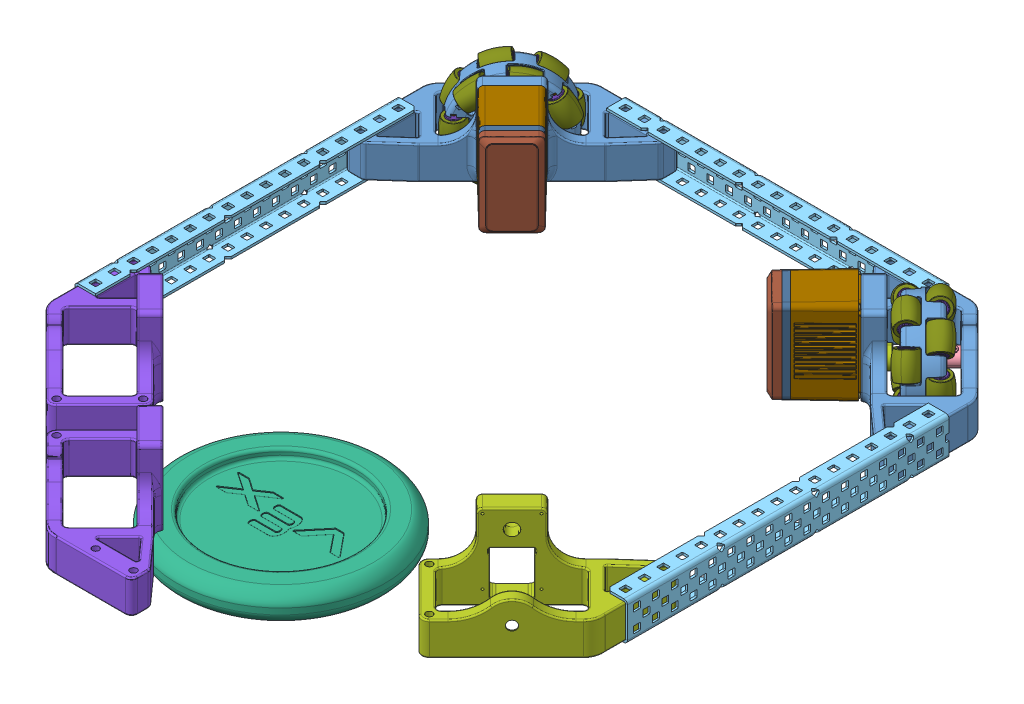
SolidWorks assembly V1_Full_Test_Fit, configuration Default. Lengths in mm.
Overall size (423.31 97.03 435.93).
184 component instances, 26 part files, 36 mates.
Components (placement in the parent):
- holo_bracket_v1_testfit-3: holo_bracket_v1_testfit [Default] at (-45.956 136.7873 -156.7355) x (0.707107 0 -0.707107) z (0.707107 0 0.707107) size (156.42 97.03 100.21)
  - holo_bracket_v2-1: holo_bracket_v2 [Default] at (-4.6322 -25.0688 0.2151) size (156.42 56.7 55.6)
  - V5 Smart Motor (276-4840) no cap-1: V5 Smart Motor (276-4840) no cap [Default] at (-4.6322 6.6812 47.4651) x (0 -1 0) z (0 0 -1) size (59.01 35.33 59.91)
    - V5 Smart Motor (276-4840).step-1: V5 Smart Motor (276-4840).step [Default] at origin size (59.01 35.33 59.91)
      - 276-4840-900 Rev6_Instruction.step-1: 276-4840-900 Rev6_Instruction.step [Default] at (-14.3 0 -17.2) size (52.79 15.94 38.15)
        - 276-4840-901 Rev6.step-1: 276-4840-901 Rev6.step [Default] at (10.75 -10.05 17.8) x (-1 0 0) z (0 0 1) size (49.9 1.6 38.15)
        - 276-4840-902 Rev2.step-1: 276-4840-902 Rev2.step [Default] at (31.25 -9.25 6.2) x (0 0 -1) z (0 -1 0) size (10.35 11.39 15.94)
        - 276-4840-022 Rev4.step-1: 276-4840-022 Rev4.step [Default] at (31.25 -9.25 6.2) x (0 0 -1) z (1 0 0) size (10.26 9.1 5.51)
      - 276-4840-110 Rev10_Instruction.step-1: 276-4840-110 Rev10_Instruction.step [Default] at (12.7 0 14.7) size (35.33 35.33 31.1)
        - 276-4840-061 Rev7_Ring_Gear_Fixed01 .6 Rev3.step-1: 276-4840-061 Rev7_Ring_Gear_Fixed01 .6 Rev3.step [Default] at origin size (28.79 28.39 24.6)
        - 276-4840-018 Rev6.step-1: 276-4840-018 Rev6.step [Default] at (0 0 6.7) x (-0.483174 0.875524 0) z (0 0 1) size (26 26 12.3)
        - 276-4840-059 Rev2.step-1: 276-4840-059 Rev2.step [Default] at (0 0 10.3) size (28.4 28.4 8.5)
        - 276-4840-062 Rev1.step-1: 276-4840-062 Rev1.step [Default] at (-12.1353 8.8168 12.3) x (0.956835 -0.290632 0) z (-0.290632 -0.956835 0) size (3.2 6.56 3.2)
        - 276-4840-062 Rev1.step-2: 276-4840-062 Rev1.step [Default] at (12.1353 8.8168 12.3) x (0.978427 0.206591 0) z (0.206591 -0.978427 0) size (3.2 6.56 3.2)
        - 276-4840-062 Rev1.step-3: 276-4840-062 Rev1.step [Default] at (-12.1353 -8.8168 12.3) x (0.72563 0.688086 0) z (0.688086 -0.72563 0) size (3.2 6.56 3.2)
      - 276-4840-001 Rev38.step-1: 276-4840-001 Rev38.step [Default] at origin size (57.3 33 46.9)
      - 276-4840-005 Rev27.step-1: 276-4840-005 Rev27.step [Default] at (0 0 -17.95) size (56.17 31.87 12.9)
      - 276-4840-004 Rev16.step-1: 276-4840-004 Rev16.step [Default] at (0 0 -19.2) size (56.01 31.71 9.21)
      - 276-4840-009 Rev3.step-1: 276-4840-009 Rev3.step [Default] at (25.45 13.5 15.7) x (0.19987 -0.979823 0) z (-0.979823 -0.19987 0) size (3.4 41.31 4.34)
      - 276-4840-009 Rev3.step-2: 276-4840-009 Rev3.step [Default] at (-25.45 -13.5 15.7) x (-0.998855 0.047836 0) z (0.047836 0.998855 0) size (3.4 41.31 4.34)
      - 276-4840-009 Rev3.step-3: 276-4840-009 Rev3.step [Default] at (25.45 -13.5 15.7) x (-0.975374 0.220559 0) z (0.220559 0.975374 0) size (3.4 41.31 4.34)
      - 276-4840-009 Rev3.step-4: 276-4840-009 Rev3.step [Default] at (-25.45 13.5 15.7) x (-0.922256 0.38658 0) z (0.38658 0.922256 0) size (3.4 41.31 4.34)
      - 276-4840-025 Rev19.step-1: 276-4840-025 Rev19.step [Default] at (12.7 0 -22.63) x (-0.993315 0.115437 0) z (0 0 1) size (14.82 14.83 35.18)
  - 0.375_ ID x 0.875_ OD x 0.281_ WD (Radial Bearing) (217-3239)-1: 0.375_ ID x 0.875_ OD x 0.281_ WD (Radial Bearing) (217-3239) [Default] at (-4.6322 -6.0188 -24.4723) x (0 0 1) z (-1 0 0) size (7.14 22.23 22.23)
  - 0.375in_ID_Bearing_Insert-1: 0.375in_ID_Bearing_Insert [Default] at (-4.6322 -6.0188 -24.4723) size (9.4 9.4 7.14)
  - 2.75 Omni with inserts (276-1902) -1: 2.75 Omni with inserts (276-1902)  [Default] at (46.131 17.9191 -68.0616) x (-0.794609 0.607122 0) z (0 0 1) size (87.15 87.98 47.75)
    - 2.75 Omni-Directional Wheel - Double Roller (276-1902) -1: 2.75 Omni-Directional Wheel - Double Roller (276-1902)  [Default] at (25.8037 49.8406 68.5807) size (87.15 87.98 47.75)
      - 2.75 Omni-Directional Wheel - Double Roller (276-1902) .step-1: 2.75 Omni-Directional Wheel - Double Roller (276-1902) .step [Default] at origin size (87.15 87.98 47.75)
        - 276-1902-010 Rev1.step-1: 276-1902-010 Rev1.step [Default] at (0 27.5 8) x (1 0 0) z (0 0.828233 0.560383) size (23 27.81 20.35)
          - 276-1902-011 Rev1.step-1: 276-1902-011 Rev1.step [Default] at (0 -6.325 -26.7627) x (1 0 0) z (0 -0.973191 0.23) size (16.5 15 25.03)
          - 276-1902-012 Rev1.step-1: 276-1902-012 Rev1.step [Default] at origin size (17.5 10.34 18.34)
          - 276-1902-003 Rev1.step-1: 276-1902-003 Rev1.step [Default] x (0 -0.928523 0.371275) z (1 0 0) size (2 2 23)
        - 276-1902-010 Rev1.step-2: 276-1902-010 Rev1.step [Default] at (0 -27.5 -8) x (1 0 0) z (0 0.410464 0.911877) size (23 27.81 20.35)
          - 276-1902-011 Rev1.step-1: 276-1902-011 Rev1.step [Default] at (0 -6.325 -26.7627) x (1 0 0) z (0 -0.973191 0.23) size (16.5 15 25.03)
          - 276-1902-012 Rev1.step-1: 276-1902-012 Rev1.step [Default] at origin size (17.5 10.34 18.34)
          - 276-1902-003 Rev1.step-1: 276-1902-003 Rev1.step [Default] x (0 -0.928523 0.371275) z (1 0 0) size (2 2 23)
        - 276-1902-010 Rev1.step-3: 276-1902-010 Rev1.step [Default] at (-21.5004 -17.146 -8) x (0.62349 -0.781831 0) z (0.320913 0.25592 0.911877) size (23 27.81 20.35)
          - 276-1902-011 Rev1.step-1: 276-1902-011 Rev1.step [Default] at (0 -6.325 -26.7627) x (1 0 0) z (0 -0.973191 0.23) size (16.5 15 25.03)
          - 276-1902-012 Rev1.step-1: 276-1902-012 Rev1.step [Default] at origin size (17.5 10.34 18.34)
          - 276-1902-003 Rev1.step-1: 276-1902-003 Rev1.step [Default] x (0 -0.928523 0.371275) z (1 0 0) size (2 2 23)
        - 276-1902-010 Rev1.step-4: 276-1902-010 Rev1.step [Default] at (-26.8105 6.1193 -8) x (-0.222521 -0.974928 0) z (0.400172 -0.091337 0.911877) size (23 27.81 20.35)
          - 276-1902-011 Rev1.step-1: 276-1902-011 Rev1.step [Default] at (0 -6.325 -26.7627) x (1 0 0) z (0 -0.973191 0.23) size (16.5 15 25.03)
          - 276-1902-012 Rev1.step-1: 276-1902-012 Rev1.step [Default] at origin size (17.5 10.34 18.34)
          - 276-1902-003 Rev1.step-1: 276-1902-003 Rev1.step [Default] x (0 -0.928523 0.371275) z (1 0 0) size (2 2 23)
        - 276-1902-010 Rev1.step-5: 276-1902-010 Rev1.step [Default] at (-11.9318 24.7766 -8) x (-0.900969 -0.433884 0) z (0.178093 -0.369815 0.911877) size (23 27.81 20.35)
          - 276-1902-011 Rev1.step-1: 276-1902-011 Rev1.step [Default] at (0 -6.325 -26.7627) x (1 0 0) z (0 -0.973191 0.23) size (16.5 15 25.03)
          - 276-1902-012 Rev1.step-1: 276-1902-012 Rev1.step [Default] at origin size (17.5 10.34 18.34)
          - 276-1902-003 Rev1.step-1: 276-1902-003 Rev1.step [Default] x (0 -0.928523 0.371275) z (1 0 0) size (2 2 23)
        - 276-1902-010 Rev1.step-6: 276-1902-010 Rev1.step [Default] at (11.9318 24.7766 -8) x (-0.900969 0.433884 0) z (-0.178093 -0.369815 0.911877) size (23 27.81 20.35)
          - 276-1902-011 Rev1.step-1: 276-1902-011 Rev1.step [Default] at (0 -6.325 -26.7627) x (1 0 0) z (0 -0.973191 0.23) size (16.5 15 25.03)
          - 276-1902-012 Rev1.step-1: 276-1902-012 Rev1.step [Default] at origin size (17.5 10.34 18.34)
          - 276-1902-003 Rev1.step-1: 276-1902-003 Rev1.step [Default] x (0 -0.928523 0.371275) z (1 0 0) size (2 2 23)
        - 276-1902-010 Rev1.step-7: 276-1902-010 Rev1.step [Default] at (26.8105 6.1193 -8) x (-0.222521 0.974928 0) z (-0.400172 -0.091337 0.911877) size (23 27.81 20.35)
          - 276-1902-011 Rev1.step-1: 276-1902-011 Rev1.step [Default] at (0 -6.325 -26.7627) x (1 0 0) z (0 -0.973191 0.23) size (16.5 15 25.03)
          - 276-1902-012 Rev1.step-1: 276-1902-012 Rev1.step [Default] at origin size (17.5 10.34 18.34)
          - 276-1902-003 Rev1.step-1: 276-1902-003 Rev1.step [Default] x (0 -0.928523 0.371275) z (1 0 0) size (2 2 23)
        - 276-1902-010 Rev1.step-8: 276-1902-010 Rev1.step [Default] at (21.5004 -17.146 -8) x (0.62349 0.781831 0) z (-0.320913 0.25592 0.911877) size (23 27.81 20.35)
          - 276-1902-011 Rev1.step-1: 276-1902-011 Rev1.step [Default] at (0 -6.325 -26.7627) x (1 0 0) z (0 -0.973191 0.23) size (16.5 15 25.03)
          - 276-1902-012 Rev1.step-1: 276-1902-012 Rev1.step [Default] at origin size (17.5 10.34 18.34)
          - 276-1902-003 Rev1.step-1: 276-1902-003 Rev1.step [Default] x (0 -0.928523 0.371275) z (1 0 0) size (2 2 23)
        - 276-1902-010 Rev1.step-9: 276-1902-010 Rev1.step [Default] at (21.5004 17.146 8) x (0.62349 -0.781831 0) z (0.647539 0.516395 0.560383) size (23 27.81 20.35)
          - 276-1902-011 Rev1.step-1: 276-1902-011 Rev1.step [Default] at (0 -6.325 -26.7627) x (1 0 0) z (0 -0.973191 0.23) size (16.5 15 25.03)
          - 276-1902-012 Rev1.step-1: 276-1902-012 Rev1.step [Default] at origin size (17.5 10.34 18.34)
          - 276-1902-003 Rev1.step-1: 276-1902-003 Rev1.step [Default] x (0 -0.928523 0.371275) z (1 0 0) size (2 2 23)
        - 276-1902-010 Rev1.step-10: 276-1902-010 Rev1.step [Default] at (26.8105 -6.1193 8) x (-0.222521 -0.974928 0) z (0.807468 -0.184299 0.560383) size (23 27.81 20.35)
          - 276-1902-011 Rev1.step-1: 276-1902-011 Rev1.step [Default] at (0 -6.325 -26.7627) x (1 0 0) z (0 -0.973191 0.23) size (16.5 15 25.03)
          - 276-1902-012 Rev1.step-1: 276-1902-012 Rev1.step [Default] at origin size (17.5 10.34 18.34)
          - 276-1902-003 Rev1.step-1: 276-1902-003 Rev1.step [Default] x (0 -0.928523 0.371275) z (1 0 0) size (2 2 23)
        - 276-1902-010 Rev1.step-11: 276-1902-010 Rev1.step [Default] at (11.9318 -24.7766 8) x (-0.900969 -0.433884 0) z (0.359357 -0.746212 0.560383) size (23 27.81 20.35)
          - 276-1902-011 Rev1.step-1: 276-1902-011 Rev1.step [Default] at (0 -6.325 -26.7627) x (1 0 0) z (0 -0.973191 0.23) size (16.5 15 25.03)
          - 276-1902-012 Rev1.step-1: 276-1902-012 Rev1.step [Default] at origin size (17.5 10.34 18.34)
          - 276-1902-003 Rev1.step-1: 276-1902-003 Rev1.step [Default] x (0 -0.928523 0.371275) z (1 0 0) size (2 2 23)
        - 276-1902-010 Rev1.step-12: 276-1902-010 Rev1.step [Default] at (-11.9318 -24.7766 8) x (-0.900969 0.433884 0) z (-0.359357 -0.746212 0.560383) size (23 27.81 20.35)
          - 276-1902-011 Rev1.step-1: 276-1902-011 Rev1.step [Default] at (0 -6.325 -26.7627) x (1 0 0) z (0 -0.973191 0.23) size (16.5 15 25.03)
          - 276-1902-012 Rev1.step-1: 276-1902-012 Rev1.step [Default] at origin size (17.5 10.34 18.34)
          - 276-1902-003 Rev1.step-1: 276-1902-003 Rev1.step [Default] x (0 -0.928523 0.371275) z (1 0 0) size (2 2 23)
        - 276-1902-010 Rev1.step-13: 276-1902-010 Rev1.step [Default] at (-26.8105 -6.1193 8) x (-0.222521 0.974928 0) z (-0.807468 -0.184299 0.560383) size (23 27.81 20.35)
          - 276-1902-011 Rev1.step-1: 276-1902-011 Rev1.step [Default] at (0 -6.325 -26.7627) x (1 0 0) z (0 -0.973191 0.23) size (16.5 15 25.03)
          - 276-1902-012 Rev1.step-1: 276-1902-012 Rev1.step [Default] at origin size (17.5 10.34 18.34)
          - 276-1902-003 Rev1.step-1: 276-1902-003 Rev1.step [Default] x (0 -0.928523 0.371275) z (1 0 0) size (2 2 23)
        - 276-1902-010 Rev1.step-14: 276-1902-010 Rev1.step [Default] at (-21.5004 17.146 8) x (0.62349 0.781831 0) z (-0.647539 0.516395 0.560383) size (23 27.81 20.35)
          - 276-1902-011 Rev1.step-1: 276-1902-011 Rev1.step [Default] at (0 -6.325 -26.7627) x (1 0 0) z (0 -0.973191 0.23) size (16.5 15 25.03)
          - 276-1902-012 Rev1.step-1: 276-1902-012 Rev1.step [Default] at origin size (17.5 10.34 18.34)
          - 276-1902-003 Rev1.step-1: 276-1902-003 Rev1.step [Default] x (0 -0.928523 0.371275) z (1 0 0) size (2 2 23)
        - 276-1902-002 Rev3.step-1: 276-1902-002 Rev3.step [Default] at origin size (66.55 66.02 25.07)
    - Metal Shaft Inserts (276-3881-002)-1: Metal Shaft Inserts (276-3881-002) [Default] at (25.8037 49.8406 79.8307) x (0 -1 0) z (1 0 0) size (10.03 5.08 10.03)
    - Metal Shaft Inserts (276-3881-002)-2: Metal Shaft Inserts (276-3881-002) [Default] at (25.8037 49.8406 57.3307) x (1 0 0) z (0 -1 0) size (10.03 5.08 10.03)
  - Drive Shaft 2in-1: Drive Shaft 2in [Default] at (-4.6322 -6.0188 -126.7349) size (3.28 3.28 50.8)
  - Shaft Collar (276-2010)-1: Shaft Collar (276-2010) [Default] at (-4.6322 -6.0188 -14.0329) x (0.96656 -0.256441 0) z (0 0 -1) size (11 11.35 6.6)
- holo_bracket_v1_testfit-4: holo_bracket_v1_testfit [Default] at (230.9219 136.7873 -150.1846) x (0.707107 0 0.707107) z (-0.707107 0 0.707107) size (156.42 97.03 100.21)
  - holo_bracket_v2-1: holo_bracket_v2 [Default] at (-4.6322 -25.0688 0.2151) size (156.42 56.7 55.6)
  - V5 Smart Motor (276-4840) no cap-1: V5 Smart Motor (276-4840) no cap [Default] at (-4.6322 6.6812 47.4651) x (0 -1 0) z (0 0 -1) size (59.01 35.33 59.91)
    - V5 Smart Motor (276-4840).step-1: V5 Smart Motor (276-4840).step [Default] at origin size (59.01 35.33 59.91)
      - 276-4840-900 Rev6_Instruction.step-1: 276-4840-900 Rev6_Instruction.step [Default] at (-14.3 0 -17.2) size (52.79 15.94 38.15)
        - 276-4840-901 Rev6.step-1: 276-4840-901 Rev6.step [Default] at (10.75 -10.05 17.8) x (-1 0 0) z (0 0 1) size (49.9 1.6 38.15)
        - 276-4840-902 Rev2.step-1: 276-4840-902 Rev2.step [Default] at (31.25 -9.25 6.2) x (0 0 -1) z (0 -1 0) size (10.35 11.39 15.94)
        - 276-4840-022 Rev4.step-1: 276-4840-022 Rev4.step [Default] at (31.25 -9.25 6.2) x (0 0 -1) z (1 0 0) size (10.26 9.1 5.51)
      - 276-4840-110 Rev10_Instruction.step-1: 276-4840-110 Rev10_Instruction.step [Default] at (12.7 0 14.7) size (35.33 35.33 31.1)
        - 276-4840-061 Rev7_Ring_Gear_Fixed01 .6 Rev3.step-1: 276-4840-061 Rev7_Ring_Gear_Fixed01 .6 Rev3.step [Default] at origin size (28.79 28.39 24.6)
        - 276-4840-018 Rev6.step-1: 276-4840-018 Rev6.step [Default] at (0 0 6.7) x (-0.483174 0.875524 0) z (0 0 1) size (26 26 12.3)
        - 276-4840-059 Rev2.step-1: 276-4840-059 Rev2.step [Default] at (0 0 10.3) size (28.4 28.4 8.5)
        - 276-4840-062 Rev1.step-1: 276-4840-062 Rev1.step [Default] at (-12.1353 8.8168 12.3) x (0.956835 -0.290632 0) z (-0.290632 -0.956835 0) size (3.2 6.56 3.2)
        - 276-4840-062 Rev1.step-2: 276-4840-062 Rev1.step [Default] at (12.1353 8.8168 12.3) x (0.978427 0.206591 0) z (0.206591 -0.978427 0) size (3.2 6.56 3.2)
        - 276-4840-062 Rev1.step-3: 276-4840-062 Rev1.step [Default] at (-12.1353 -8.8168 12.3) x (0.72563 0.688086 0) z (0.688086 -0.72563 0) size (3.2 6.56 3.2)
      - 276-4840-001 Rev38.step-1: 276-4840-001 Rev38.step [Default] at origin size (57.3 33 46.9)
      - 276-4840-005 Rev27.step-1: 276-4840-005 Rev27.step [Default] at (0 0 -17.95) size (56.17 31.87 12.9)
      - 276-4840-004 Rev16.step-1: 276-4840-004 Rev16.step [Default] at (0 0 -19.2) size (56.01 31.71 9.21)
      - 276-4840-009 Rev3.step-1: 276-4840-009 Rev3.step [Default] at (25.45 13.5 15.7) x (0.19987 -0.979823 0) z (-0.979823 -0.19987 0) size (3.4 41.31 4.34)
      - 276-4840-009 Rev3.step-2: 276-4840-009 Rev3.step [Default] at (-25.45 -13.5 15.7) x (-0.998855 0.047836 0) z (0.047836 0.998855 0) size (3.4 41.31 4.34)
      - 276-4840-009 Rev3.step-3: 276-4840-009 Rev3.step [Default] at (25.45 -13.5 15.7) x (-0.975374 0.220559 0) z (0.220559 0.975374 0) size (3.4 41.31 4.34)
      - 276-4840-009 Rev3.step-4: 276-4840-009 Rev3.step [Default] at (-25.45 13.5 15.7) x (-0.922256 0.38658 0) z (0.38658 0.922256 0) size (3.4 41.31 4.34)
      - 276-4840-025 Rev19.step-1: 276-4840-025 Rev19.step [Default] at (12.7 0 -22.63) x (-0.993315 0.115437 0) z (0 0 1) size (14.82 14.83 35.18)
  - 0.375_ ID x 0.875_ OD x 0.281_ WD (Radial Bearing) (217-3239)-1: 0.375_ ID x 0.875_ OD x 0.281_ WD (Radial Bearing) (217-3239) [Default] at (-4.6322 -6.0188 -24.4723) x (0 0 1) z (-1 0 0) size (7.14 22.23 22.23)
  - 0.375in_ID_Bearing_Insert-1: 0.375in_ID_Bearing_Insert [Default] at (-4.6322 -6.0188 -24.4723) size (9.4 9.4 7.14)
  - 2.75 Omni with inserts (276-1902) -1: 2.75 Omni with inserts (276-1902)  [Default] at (46.131 17.9191 -68.0616) x (-0.794609 0.607122 0) z (0 0 1) size (87.15 87.98 47.75)
    - 2.75 Omni-Directional Wheel - Double Roller (276-1902) -1: 2.75 Omni-Directional Wheel - Double Roller (276-1902)  [Default] at (25.8037 49.8406 68.5807) size (87.15 87.98 47.75)
      - 2.75 Omni-Directional Wheel - Double Roller (276-1902) .step-1: 2.75 Omni-Directional Wheel - Double Roller (276-1902) .step [Default] at origin size (87.15 87.98 47.75)
        - 276-1902-010 Rev1.step-1: 276-1902-010 Rev1.step [Default] at (0 27.5 8) x (1 0 0) z (0 0.828233 0.560383) size (23 27.81 20.35)
          - 276-1902-011 Rev1.step-1: 276-1902-011 Rev1.step [Default] at (0 -6.325 -26.7627) x (1 0 0) z (0 -0.973191 0.23) size (16.5 15 25.03)
          - 276-1902-012 Rev1.step-1: 276-1902-012 Rev1.step [Default] at origin size (17.5 10.34 18.34)
          - 276-1902-003 Rev1.step-1: 276-1902-003 Rev1.step [Default] x (0 -0.928523 0.371275) z (1 0 0) size (2 2 23)
        - 276-1902-010 Rev1.step-2: 276-1902-010 Rev1.step [Default] at (0 -27.5 -8) x (1 0 0) z (0 0.410464 0.911877) size (23 27.81 20.35)
          - 276-1902-011 Rev1.step-1: 276-1902-011 Rev1.step [Default] at (0 -6.325 -26.7627) x (1 0 0) z (0 -0.973191 0.23) size (16.5 15 25.03)
          - 276-1902-012 Rev1.step-1: 276-1902-012 Rev1.step [Default] at origin size (17.5 10.34 18.34)
          - 276-1902-003 Rev1.step-1: 276-1902-003 Rev1.step [Default] x (0 -0.928523 0.371275) z (1 0 0) size (2 2 23)
        - 276-1902-010 Rev1.step-3: 276-1902-010 Rev1.step [Default] at (-21.5004 -17.146 -8) x (0.62349 -0.781831 0) z (0.320913 0.25592 0.911877) size (23 27.81 20.35)
          - 276-1902-011 Rev1.step-1: 276-1902-011 Rev1.step [Default] at (0 -6.325 -26.7627) x (1 0 0) z (0 -0.973191 0.23) size (16.5 15 25.03)
          - 276-1902-012 Rev1.step-1: 276-1902-012 Rev1.step [Default] at origin size (17.5 10.34 18.34)
          - 276-1902-003 Rev1.step-1: 276-1902-003 Rev1.step [Default] x (0 -0.928523 0.371275) z (1 0 0) size (2 2 23)
        - 276-1902-010 Rev1.step-4: 276-1902-010 Rev1.step [Default] at (-26.8105 6.1193 -8) x (-0.222521 -0.974928 0) z (0.400172 -0.091337 0.911877) size (23 27.81 20.35)
          - 276-1902-011 Rev1.step-1: 276-1902-011 Rev1.step [Default] at (0 -6.325 -26.7627) x (1 0 0) z (0 -0.973191 0.23) size (16.5 15 25.03)
          - 276-1902-012 Rev1.step-1: 276-1902-012 Rev1.step [Default] at origin size (17.5 10.34 18.34)
          - 276-1902-003 Rev1.step-1: 276-1902-003 Rev1.step [Default] x (0 -0.928523 0.371275) z (1 0 0) size (2 2 23)
        - 276-1902-010 Rev1.step-5: 276-1902-010 Rev1.step [Default] at (-11.9318 24.7766 -8) x (-0.900969 -0.433884 0) z (0.178093 -0.369815 0.911877) size (23 27.81 20.35)
          - 276-1902-011 Rev1.step-1: 276-1902-011 Rev1.step [Default] at (0 -6.325 -26.7627) x (1 0 0) z (0 -0.973191 0.23) size (16.5 15 25.03)
          - 276-1902-012 Rev1.step-1: 276-1902-012 Rev1.step [Default] at origin size (17.5 10.34 18.34)
          - 276-1902-003 Rev1.step-1: 276-1902-003 Rev1.step [Default] x (0 -0.928523 0.371275) z (1 0 0) size (2 2 23)
        - 276-1902-010 Rev1.step-6: 276-1902-010 Rev1.step [Default] at (11.9318 24.7766 -8) x (-0.900969 0.433884 0) z (-0.178093 -0.369815 0.911877) size (23 27.81 20.35)
          - 276-1902-011 Rev1.step-1: 276-1902-011 Rev1.step [Default] at (0 -6.325 -26.7627) x (1 0 0) z (0 -0.973191 0.23) size (16.5 15 25.03)
          - 276-1902-012 Rev1.step-1: 276-1902-012 Rev1.step [Default] at origin size (17.5 10.34 18.34)
          - 276-1902-003 Rev1.step-1: 276-1902-003 Rev1.step [Default] x (0 -0.928523 0.371275) z (1 0 0) size (2 2 23)
        - 276-1902-010 Rev1.step-7: 276-1902-010 Rev1.step [Default] at (26.8105 6.1193 -8) x (-0.222521 0.974928 0) z (-0.400172 -0.091337 0.911877) size (23 27.81 20.35)
          - 276-1902-011 Rev1.step-1: 276-1902-011 Rev1.step [Default] at (0 -6.325 -26.7627) x (1 0 0) z (0 -0.973191 0.23) size (16.5 15 25.03)
          - 276-1902-012 Rev1.step-1: 276-1902-012 Rev1.step [Default] at origin size (17.5 10.34 18.34)
          - 276-1902-003 Rev1.step-1: 276-1902-003 Rev1.step [Default] x (0 -0.928523 0.371275) z (1 0 0) size (2 2 23)
        - 276-1902-010 Rev1.step-8: 276-1902-010 Rev1.step [Default] at (21.5004 -17.146 -8) x (0.62349 0.781831 0) z (-0.320913 0.25592 0.911877) size (23 27.81 20.35)
          - 276-1902-011 Rev1.step-1: 276-1902-011 Rev1.step [Default] at (0 -6.325 -26.7627) x (1 0 0) z (0 -0.973191 0.23) size (16.5 15 25.03)
          - 276-1902-012 Rev1.step-1: 276-1902-012 Rev1.step [Default] at origin size (17.5 10.34 18.34)
          - 276-1902-003 Rev1.step-1: 276-1902-003 Rev1.step [Default] x (0 -0.928523 0.371275) z (1 0 0) size (2 2 23)
        - 276-1902-010 Rev1.step-9: 276-1902-010 Rev1.step [Default] at (21.5004 17.146 8) x (0.62349 -0.781831 0) z (0.647539 0.516395 0.560383) size (23 27.81 20.35)
          - 276-1902-011 Rev1.step-1: 276-1902-011 Rev1.step [Default] at (0 -6.325 -26.7627) x (1 0 0) z (0 -0.973191 0.23) size (16.5 15 25.03)
          - 276-1902-012 Rev1.step-1: 276-1902-012 Rev1.step [Default] at origin size (17.5 10.34 18.34)
          - 276-1902-003 Rev1.step-1: 276-1902-003 Rev1.step [Default] x (0 -0.928523 0.371275) z (1 0 0) size (2 2 23)
        - 276-1902-010 Rev1.step-10: 276-1902-010 Rev1.step [Default] at (26.8105 -6.1193 8) x (-0.222521 -0.974928 0) z (0.807468 -0.184299 0.560383) size (23 27.81 20.35)
          - 276-1902-011 Rev1.step-1: 276-1902-011 Rev1.step [Default] at (0 -6.325 -26.7627) x (1 0 0) z (0 -0.973191 0.23) size (16.5 15 25.03)
          - 276-1902-012 Rev1.step-1: 276-1902-012 Rev1.step [Default] at origin size (17.5 10.34 18.34)
          - 276-1902-003 Rev1.step-1: 276-1902-003 Rev1.step [Default] x (0 -0.928523 0.371275) z (1 0 0) size (2 2 23)
        - 276-1902-010 Rev1.step-11: 276-1902-010 Rev1.step [Default] at (11.9318 -24.7766 8) x (-0.900969 -0.433884 0) z (0.359357 -0.746212 0.560383) size (23 27.81 20.35)
          - 276-1902-011 Rev1.step-1: 276-1902-011 Rev1.step [Default] at (0 -6.325 -26.7627) x (1 0 0) z (0 -0.973191 0.23) size (16.5 15 25.03)
          - 276-1902-012 Rev1.step-1: 276-1902-012 Rev1.step [Default] at origin size (17.5 10.34 18.34)
          - 276-1902-003 Rev1.step-1: 276-1902-003 Rev1.step [Default] x (0 -0.928523 0.371275) z (1 0 0) size (2 2 23)
        - 276-1902-010 Rev1.step-12: 276-1902-010 Rev1.step [Default] at (-11.9318 -24.7766 8) x (-0.900969 0.433884 0) z (-0.359357 -0.746212 0.560383) size (23 27.81 20.35)
          - 276-1902-011 Rev1.step-1: 276-1902-011 Rev1.step [Default] at (0 -6.325 -26.7627) x (1 0 0) z (0 -0.973191 0.23) size (16.5 15 25.03)
          - 276-1902-012 Rev1.step-1: 276-1902-012 Rev1.step [Default] at origin size (17.5 10.34 18.34)
          - 276-1902-003 Rev1.step-1: 276-1902-003 Rev1.step [Default] x (0 -0.928523 0.371275) z (1 0 0) size (2 2 23)
        - 276-1902-010 Rev1.step-13: 276-1902-010 Rev1.step [Default] at (-26.8105 -6.1193 8) x (-0.222521 0.974928 0) z (-0.807468 -0.184299 0.560383) size (23 27.81 20.35)
          - 276-1902-011 Rev1.step-1: 276-1902-011 Rev1.step [Default] at (0 -6.325 -26.7627) x (1 0 0) z (0 -0.973191 0.23) size (16.5 15 25.03)
          - 276-1902-012 Rev1.step-1: 276-1902-012 Rev1.step [Default] at origin size (17.5 10.34 18.34)
          - 276-1902-003 Rev1.step-1: 276-1902-003 Rev1.step [Default] x (0 -0.928523 0.371275) z (1 0 0) size (2 2 23)
        - 276-1902-010 Rev1.step-14: 276-1902-010 Rev1.step [Default] at (-21.5004 17.146 8) x (0.62349 0.781831 0) z (-0.647539 0.516395 0.560383) size (23 27.81 20.35)
          - 276-1902-011 Rev1.step-1: 276-1902-011 Rev1.step [Default] at (0 -6.325 -26.7627) x (1 0 0) z (0 -0.973191 0.23) size (16.5 15 25.03)
          - 276-1902-012 Rev1.step-1: 276-1902-012 Rev1.step [Default] at origin size (17.5 10.34 18.34)
          - 276-1902-003 Rev1.step-1: 276-1902-003 Rev1.step [Default] x (0 -0.928523 0.371275) z (1 0 0) size (2 2 23)
        - 276-1902-002 Rev3.step-1: 276-1902-002 Rev3.step [Default] at origin size (66.55 66.02 25.07)
    - Metal Shaft Inserts (276-3881-002)-1: Metal Shaft Inserts (276-3881-002) [Default] at (25.8037 49.8406 79.8307) x (0 -1 0) z (1 0 0) size (10.03 5.08 10.03)
    - Metal Shaft Inserts (276-3881-002)-2: Metal Shaft Inserts (276-3881-002) [Default] at (25.8037 49.8406 57.3307) x (1 0 0) z (0 -1 0) size (10.03 5.08 10.03)
  - Drive Shaft 2in-1: Drive Shaft 2in [Default] at (-4.6322 -6.0188 -126.7349) size (3.28 3.28 50.8)
  - Shaft Collar (276-2010)-1: Shaft Collar (276-2010) [Default] at (-4.6322 -6.0188 -14.0329) x (0.96656 -0.256441 0) z (0 0 -1) size (11 11.35 6.6)
- 1x2x1x17 Aluminum C-Channel-1: 1x2x1x17 Aluminum C-Channel [Default] at (-96.2125 122.8434 99.2789) x (0 0 1) z (-1 0 0) size (215.9 25.41 13.97)
- 1x2x1x17 Aluminum C-Channel-2: 1x2x1x17 Aluminum C-Channel [Default] at (274.6275 122.8434 -129.3211) x (0 0 -1) z (1 0 0) size (215.9 25.41 13.97)
- 1x2x1x17 Aluminum C-Channel-3: 1x2x1x17 Aluminum C-Channel [Default] at (-25.0925 122.8434 -200.4411) x (-1 0 0) z (0 0 -1) size (215.9 25.41 13.97)
- Disk-1: Disk [Default] at (-2247.5518 87.5186 -372.0943) size (142.7 20 142.7)
- holo_bracket_v3_Left-1: holo_bracket_v3_Left [Default] at (227.4944 111.7186 123.2658) x (-0.707107 0 0.707107) z (-0.707107 0 -0.707107) size (122.41 56.7 55.6)
- holo_bracket_v3_Right-1: holo_bracket_v3_Right [Default] at (27.5639 111.7186 199.9091) x (-0.707107 0 -0.707107) z (0.707107 0 -0.707107) size (264.81 56.7 55.6)
Mates (geometry in assembly coordinates):
- Concentric13: concentric anti-aligned: cylinder of holo_bracket_v1_testfit-1/holo_bracket_v2-1 through (-88.5925 133.9682 86.5789) axis (0 -1 0) radius 2.3; circle of 1x2x1x17 Aluminum C-Channel-1
- Concentric14: concentric anti-aligned: cylinder of holo_bracket_v1_testfit-1/holo_bracket_v2-1 through (-88.5925 133.9682 61.1789) axis (0 -1 0) radius 2.3; circle of 1x2x1x17 Aluminum C-Channel-1
- Coincident7: coincident anti-aligned: plane of holo_bracket_v1_testfit-1/holo_bracket_v2-1 through (-49.0794 111.7182 123.2658) normal (0 -1 0); plane of 1x2x1x17 Aluminum C-Channel-1 through (-84.7306 111.7182 -122.4711) normal (0 1 0)
- Concentric15: concentric anti-aligned: cylinder of holo_bracket_v1_testfit-3/holo_bracket_v2-1 through (-88.5925 133.9686 -116.6211) axis (0 -1 0) radius 2.3; circle of 1x2x1x17 Aluminum C-Channel-1
- Concentric16: concentric anti-aligned: cylinder of holo_bracket_v1_testfit-3/holo_bracket_v2-1 through (-88.5925 133.9686 -91.2211) axis (0 -1 0) radius 2.3; circle of 1x2x1x17 Aluminum C-Channel-1
- Coincident8: coincident anti-aligned: plane of holo_bracket_v1_testfit-3/holo_bracket_v2-1 through (-49.0794 133.9686 -153.308) normal (0 1 0); plane of 1x2x1x17 Aluminum C-Channel-1 through (-128.5712 133.9686 -122.4711) normal (0 -1 0)
- Concentric17: concentric anti-aligned: cylinder of holo_bracket_v1_testfit-3/holo_bracket_v2-1 through (-12.3925 133.9686 -192.8211) axis (0 -1 0) radius 2.3; circle of 1x2x1x17 Aluminum C-Channel-3
- Concentric18: concentric anti-aligned: cylinder of holo_bracket_v1_testfit-3/holo_bracket_v2-1 through (13.0075 133.9686 -192.8211) axis (0 -1 0) radius 2.3; circle of 1x2x1x17 Aluminum C-Channel-3
- Coincident9: coincident anti-aligned: plane of holo_bracket_v1_testfit-3/holo_bracket_v2-1 through (-49.0794 133.9686 -153.308) normal (0 1 0); plane of 1x2x1x17 Aluminum C-Channel-3 through (196.6575 133.9686 -232.7998) normal (0 -1 0)
- Concentric19: concentric anti-aligned: cylinder of holo_bracket_v1_testfit-4/holo_bracket_v2-1 through (190.8075 133.9686 -192.8211) axis (0 -1 0) radius 2.3; circle of 1x2x1x17 Aluminum C-Channel-3
- Concentric20: concentric anti-aligned: cylinder of holo_bracket_v1_testfit-4/holo_bracket_v2-1 through (165.4075 133.9686 -192.8211) axis (0 -1 0) radius 2.3; circle of 1x2x1x17 Aluminum C-Channel-3
- Coincident10: coincident anti-aligned: plane of holo_bracket_v1_testfit-4/holo_bracket_v2-1 through (227.4944 133.9686 -153.308) normal (0 1 0); plane of 1x2x1x17 Aluminum C-Channel-3 through (196.6575 133.9686 -232.7998) normal (0 -1 0)
- Concentric21: concentric anti-aligned: cylinder of holo_bracket_v1_testfit-4/holo_bracket_v2-1 through (267.0075 133.9686 -116.6211) axis (0 -1 0) radius 2.3; circle of 1x2x1x17 Aluminum C-Channel-2
- Concentric22: concentric anti-aligned: cylinder of holo_bracket_v1_testfit-4/holo_bracket_v2-1 through (267.0075 133.9686 -91.2211) axis (0 -1 0) radius 2.3; circle of 1x2x1x17 Aluminum C-Channel-2
- Coincident11: coincident anti-aligned: plane of holo_bracket_v1_testfit-4/holo_bracket_v2-1 through (227.4944 133.9686 -153.308) normal (0 1 0); plane of 1x2x1x17 Aluminum C-Channel-2 through (306.9862 133.9686 92.4289) normal (0 -1 0)
- Coincident18: coincident anti-aligned: plane of 1x2x1x17 Aluminum C-Channel-2 through (306.9862 133.9686 92.4289) normal (0 -1 0); plane of 90degree_mount_1-1 through (267.0075 133.9686 -27.7211) normal (0 1 0)
- Concentric29: concentric anti-aligned: cylinder of 90degree_mount_1-1 through (267.0075 133.9686 -27.7211) axis (0 -1 0) radius 2.3; circle of 1x2x1x17 Aluminum C-Channel-2
- Concentric30: concentric anti-aligned: circle of 1x2x1x27 Aluminum C-Channel-1; cylinder of 90degree_mount_1-1 through (254.3075 133.9686 -2.3211) axis (0 -1 0) radius 2.3
- Concentric31: concentric anti-aligned: circle of 1x2x1x27 Aluminum C-Channel-1; cylinder of 90degree_mount_1-1 through (228.9075 133.9686 -2.3211) axis (0 -1 0) radius 2.3
- Coincident19: coincident anti-aligned: plane of 1x2x1x27 Aluminum C-Channel-1 through (-81.7425 133.9686 37.6576) normal (0 -1 0); plane of 90degree_mount_1-1 through (267.0075 133.9686 -27.7211) normal (0 1 0)
- Coincident20: coincident anti-aligned: plane of 1x2x1x17 Aluminum C-Channel-1 through (-84.7306 111.7182 -122.4711) normal (0 1 0); plane of 90degree_mount_1-2 through (-88.5925 111.7182 -27.7211) normal (0 -1 0)
- Concentric33: concentric aligned: circle of 1x2x1x27 Aluminum C-Channel-1; cylinder of 90degree_mount_1-2 through (-50.4925 111.7182 -2.3211) axis (0 1 0) radius 2.3
- Coincident26: coincident anti-aligned: plane of 1x2x1x27 Aluminum C-Channel-1 through (-81.7425 100.9231 5.2989) normal (0 0 1); plane of 1x2x1x20 Aluminum C-Channel-1 through (138.1288 110.6434 5.2989) normal (0 0 -1)
- Coincident29: coincident anti-aligned: plane of 1x2x1x27 Aluminum C-Channel-1 through (-81.7425 100.9231 5.2989) normal (0 0 1); plane of 1x2x1x20 Aluminum C-Channel-2 through (-16.2544 110.6434 5.2989) normal (0 0 -1)
- Coincident30: coincident anti-aligned: circle of 1x2x1x27 Aluminum C-Channel-1; circle of 1x2x1x20 Aluminum C-Channel-1
- Parallel1: parallel aligned: plane of 1x2x1x17 Aluminum C-Channel-2 through (274.6275 100.9231 92.4289) normal (1 0 0); plane of 1x2x1x20 Aluminum C-Channel-1 through (184.4575 112.6315 6.8737) normal (1 0 0)
- Concentric40: concentric aligned: circle of 1x2x1x20 Aluminum C-Channel-2; circle of 1x2x1x27 Aluminum C-Channel-1
- Parallel2: parallel aligned: plane of 1x2x1x17 Aluminum C-Channel-1 through (-96.2125 100.9231 -122.4711) normal (-1 0 0); plane of 1x2x1x20 Aluminum C-Channel-2 through (-18.7425 171.1553 6.8737) normal (-1 0 0)
- Parallel3: parallel aligned: plane of 1x2x1x17 Aluminum C-Channel-1 through (-96.2125 100.9231 -122.4711) normal (-1 0 0); plane of 90degree_mount_1-2 through (-92.5925 111.7182 -27.7211) normal (-1 0 0)
- Coincident31: coincident aligned: plane of Disk-1 through (87.1248 97.5186 137.9057) normal (0 -1 0)
- Coincident32: coincident anti-aligned: plane of 1x2x1x17 Aluminum C-Channel-2 through (306.9862 133.9686 92.4289) normal (0 -1 0); plane of holo_bracket_v3_Left-1 through (227.4944 133.9686 123.2658) normal (0 1 0)
- Parallel4: parallel anti-aligned: plane of 1x2x1x17 Aluminum C-Channel-2 through (273.0527 100.9231 92.4289) normal (-1 0 0); plane of holo_bracket_v3_Left-1 through (273.3575 133.9686 123.2658) normal (1 0 0)
- Concentric41: concentric anti-aligned: circle of 1x2x1x17 Aluminum C-Channel-2; cylinder of holo_bracket_v3_Left-1 through (267.0075 133.9686 86.5789) axis (0 -1 0) radius 2.3
- Coincident34: coincident anti-aligned: plane of 1x2x1x17 Aluminum C-Channel-1 through (-128.5712 133.9686 -122.4711) normal (0 -1 0); plane of holo_bracket_v3_Right-1 through (-49.0794 133.9686 123.2658) normal (0 1 0)
- Parallel5: parallel anti-aligned: plane of 1x2x1x17 Aluminum C-Channel-1 through (-94.6377 100.9231 -122.4711) normal (1 0 0); plane of holo_bracket_v3_Right-1 through (-94.9425 133.9686 123.2658) normal (-1 0 0)
- Concentric42: concentric anti-aligned: circle of 1x2x1x17 Aluminum C-Channel-1; cylinder of holo_bracket_v3_Right-1 through (-88.5925 133.9686 86.5789) axis (0 -1 0) radius 2.3
